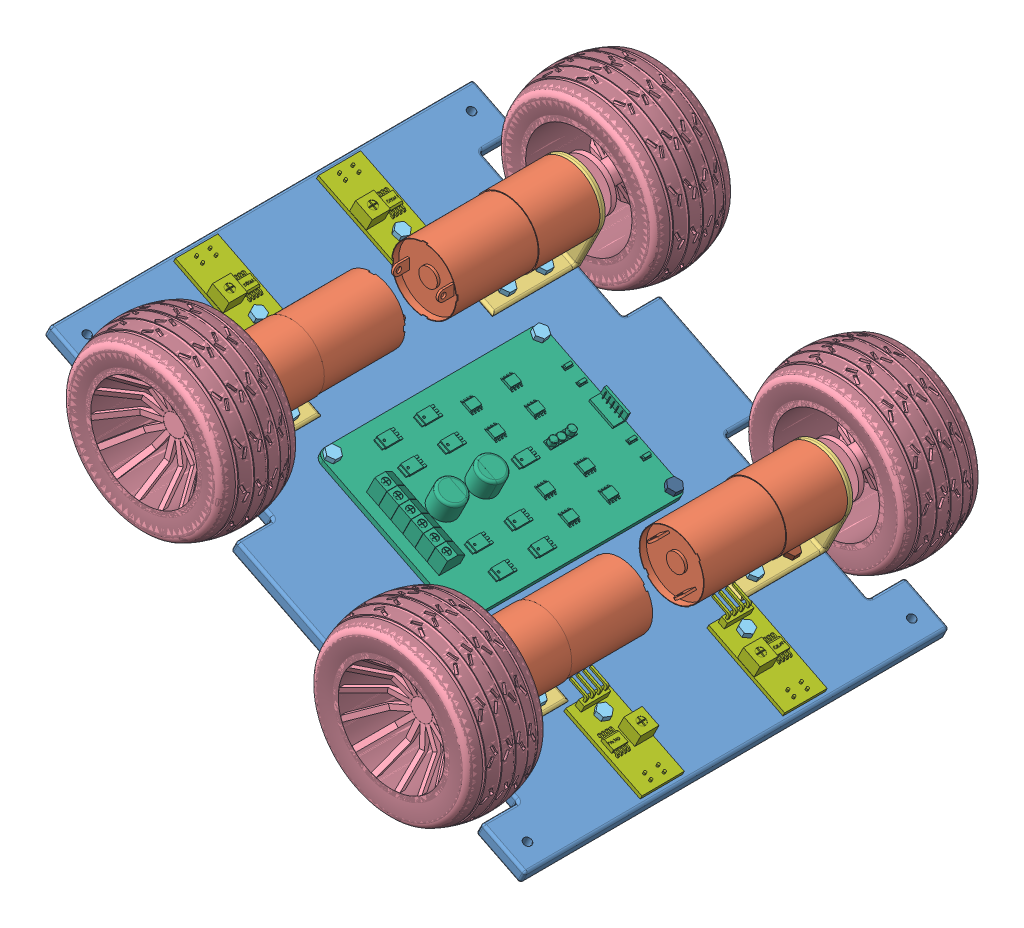
SolidWorks assembly chasse 1 assembly, configuration Default. Lengths in mm.
Overall size (204.59 144.82 194.38).
79 component instances, 12 part files, 19 mates.
Components (placement in the parent):
- down chasse-1: down chasse [Default] at (-215.8058 163.912 27.6173) x (-0.893788 0.448484 0.002276) z (-0.002035 0.001021 -0.999997) size (200 5 160)
- Motor assembly-9: Motor assembly [Default] at (-169.303 117.4456 37.7845) x (-0.59772 0.801702 0.002172) z (-0.002172 0.00109 -0.999997) size (81.67 81.67 90.74)
  - dc motor-1: dc motor [Default] at (29.3048 35.2797 20.0121) size (25 25 72.3)
  - new motor holder-1: new motor holder [Default] at (32.8529 14.4792 73.8121) x (-0.89379 0.448485 0) z (0 0 -1) size (25 31.5 33)
  - tire-2: tire [Défaut] at (29.3048 35.2797 92.3578) x (0 0 -1) z (-0.952681 -0.303972 0) size (29.78 64.99 64.99)
  - bolt-1: bolt [Default] at (36.902 31.4676 76.4477) x (-0.31031 -0.950635 0) z (0 0 -1) size (5.19 4.62 12)
  - bolt-2: bolt [Default] at (21.7075 39.0918 76.1821) x (0.923728 0.383049 0) z (0 0 -1) size (5.19 4.62 12)
- Motor assembly-14: Motor assembly [MirrorDefault] at (-169.345 117.4667 17.166) x (-0.59772 0.801703 0.001897) z (-0.001897 0.000952 -0.999998) size (81.67 81.67 90.74)
  - dc motor-1: dc motor [MirrorDefault] at (29.3048 35.2797 -20.0121) size (25 25 72.3)
  - new motor holder-1: new motor holder [MirrorDefault] at (32.8529 14.4792 -73.8121) x (-0.89379 0.448485 0) z (0 0 -1) size (25 31.5 33)
  - tire-2: tire [MirrorDéfaut] at (29.3048 35.2797 -92.3578) x (0 0 1) z (0.952681 0.303972 0) size (29.78 64.99 64.99)
  - bolt-1: bolt [MirrorDefault] at (36.902 31.4676 -76.4477) x (-0.31031 -0.950635 0) z (0 0 -1) size (5.19 4.62 12)
  - bolt-2: bolt [MirrorDefault] at (21.7075 39.0918 -76.1821) x (0.923728 0.383049 0) z (0 0 -1) size (5.19 4.62 12)
- Motor assembly-15: Motor assembly [MirrorDefault] at (-280.8119 173.3985 38.0686) x (0.999998 0.000001 -0.001897) z (0.001897 -0.000952 0.999998) size (81.67 81.67 90.74)
  - dc motor-1: dc motor [MirrorDefault] at (29.3048 35.2797 -20.0121) size (25 25 72.3)
  - new motor holder-1: new motor holder [MirrorDefault] at (32.8529 14.4792 -73.8121) x (-0.89379 0.448485 0) z (0 0 -1) size (25 31.5 33)
  - tire-2: tire [MirrorDéfaut] at (29.3048 35.2797 -92.3578) x (0 0 1) z (0.952681 0.303972 0) size (29.78 64.99 64.99)
  - bolt-1: bolt [MirrorDefault] at (36.902 31.4676 -76.4477) x (-0.31031 -0.950635 0) z (0 0 -1) size (5.19 4.62 12)
  - bolt-2: bolt [MirrorDefault] at (21.7075 39.0918 -76.1821) x (0.923728 0.383049 0) z (0 0 -1) size (5.19 4.62 12)
- Motor assembly-16: Motor assembly [MirrorMirrorDefault] at (-280.8538 173.4195 17.45) x (0.999998 0.000001 -0.002172) z (0.002172 -0.00109 0.999997) size (81.67 81.67 90.74)
  - dc motor-1: dc motor [MirrorMirrorDefault] at (29.3048 35.2797 20.0121) size (25 25 72.3)
  - new motor holder-1: new motor holder [MirrorMirrorDefault] at (32.8529 14.4792 73.8121) x (-0.89379 0.448485 0) z (0 0 -1) size (25 31.5 33)
  - tire-2: tire [MirrorMirrorDéfaut] at (29.3048 35.2797 92.3578) x (0 0 -1) z (-0.952681 -0.303972 0) size (29.78 64.99 64.99)
  - bolt-1: bolt [MirrorMirrorDefault] at (36.902 31.4676 76.4477) x (-0.31031 -0.950635 0) z (0 0 -1) size (5.19 4.62 12)
  - bolt-2: bolt [MirrorMirrorDefault] at (21.7075 39.0918 76.1821) x (0.923728 0.383049 0) z (0 0 -1) size (5.19 4.62 12)
- Motor Driver-1: Motor Driver [Default] at (-213.5634 168.381 27.6173) x (-0.002035 0.001021 -0.999997) z (0.893788 -0.448484 -0.002276) size (84.5 10.09 62)
- Arduino_HM_proximity_sensor-1: Arduino_HM_proximity_sensor [По умолчанию] at (-153.9567 140.1498 8.4513) x (0.89379 -0.448485 0.000154) z (-0.448485 -0.89379 0) size (37.02 16 16.8)
- Arduino_HM_proximity_sensor-2: Arduino_HM_proximity_sensor [MirrorПо умолчанию] at (-153.8794 140.111 46.4828) x (0.89378 -0.44848 -0.004707) z (0.448485 0.89379 0) size (37.02 16 16.8)
- Arduino_HM_proximity_sensor-3: Arduino_HM_proximity_sensor [MirrorПо умолчанию] at (-271.902 199.3323 8.7517) x (-0.89378 0.44848 0.004707) z (0.448485 0.89379 0) size (37.02 16 16.8)
- Arduino_HM_proximity_sensor-4: Arduino_HM_proximity_sensor [MirrorПо умолчанию] at (-271.8268 199.2946 62.7833) x (-0.89379 0.448485 -0.000154) z (0.448485 0.89379 0) size (37.02 16 16.8)
- Part1^chasse 1 assembly-1: Part1^chasse 1 assembly [Default] at origin (virtual)
- bolt-1: bolt [Default] at (-147.6975 138.1279 0.4523) x (-0.34547 0.17335 -0.92228) z (-0.448485 -0.89379 0) size (5.19 4.62 12)
- nut (1)-1: nut (1) [Default] at (-151.7339 130.0838 0.4523) x (0.798861 -0.400852 -0.448485) z (0.448485 0.89379 0) size (5.28 5.69 3.19)
- Mirrornut (1)-2: Mirrornut (1) [Default] at (-151.624 130.0287 54.4522) x (0.800678 -0.401763 0.444411) z (-0.448485 -0.89379 0) size (5.28 5.69 3.19)
- bolt-2: bolt [Default] at (-147.5876 138.0728 54.4522) x (-0.341714 0.171465 0.92403) z (-0.448485 -0.89379 0) size (5.19 4.62 12)
- Mirrornut (1)-3: Mirrornut (1) [Default] at (-281.3331 195.114 0.7824) x (-0.800678 0.401763 -0.444411) z (-0.448485 -0.89379 0) size (5.28 5.69 3.19)
- bolt-3: bolt [Default] at (-277.2968 203.1581 0.7824) x (0.341714 -0.171465 -0.92403) z (-0.448485 -0.89379 0) size (5.19 4.62 12)
- Mirrornut (1)-4: Mirrornut (1) [Default] at (-281.2235 195.0583 54.7823) x (-0.798861 0.400852 0.448485) z (0.448485 0.89379 0) size (5.28 5.69 3.19)
- bolt-4: bolt [Default] at (-277.1869 203.103 54.7823) x (0.34547 -0.17335 0.92228) z (-0.448485 -0.89379 0) size (5.19 4.62 12)
- bolt-5: bolt [Default] at (-237.279 183.7494 -11.5689) x (0.798861 -0.400852 0.448485) z (-0.448485 -0.89379 0) size (5.19 4.62 12)
- nut (1)-2: nut (1) [Default] at (-241.5918 175.1726 -11.4981) x (0.887126 -0.445142 0.121884) z (-0.448485 -0.89379 0) size (5.28 5.69 3.19)
- Mirrorbolt-6: Mirrorbolt [Default] at (-187.2269 158.6343 -11.6964) x (-0.797028 0.399932 0.45255) z (0.448485 0.89379 0) size (5.19 4.62 12)
- nut (1)-3: nut (1) [Default] at (-191.5245 150.0506 -11.6256) x (-0.886621 0.444888 0.126402) z (0.448485 0.89379 0) size (5.28 5.69 3.19)
- bolt-6: bolt [Default] at (-237.1193 183.6692 66.9309) x (0.797028 -0.399932 -0.45255) z (-0.448485 -0.89379 0) size (5.19 4.62 12)
- nut (1)-4: nut (1) [Default] at (-241.4321 175.0932 66.8601) x (0.886621 -0.444888 -0.126402) z (0.448485 0.89379 0) size (5.28 5.69 3.19)
- Mirrorbolt-7: Mirrorbolt [Default] at (-187.0672 158.5541 66.8034) x (-0.798861 0.400852 -0.448485) z (0.448485 0.89379 0) size (5.19 4.62 12)
- nut (1)-5: nut (1) [Default] at (-191.3654 149.9701 66.7326) x (-0.887126 0.445142 -0.121884) z (-0.448485 -0.89379 0) size (5.28 5.69 3.19)
- bolt-7: bolt [Default] at (-251.4631 190.7548 68.7173) x (0.798861 -0.400852 0.448485) z (-0.448485 -0.89379 0) size (5.19 4.62 12)
- nut (1)-6: nut (1) [Default] at (-255.7218 182.2628 68.7173) x (0.798861 -0.400852 -0.448485) z (0.448485 0.89379 0) size (5.28 5.69 3.19)
- nut (1)-7: nut (1) [Default] at (-255.6933 182.2485 82.7173) x (0.798861 -0.400852 0.448485) z (-0.448485 -0.89379 0) size (5.28 5.69 3.19)
- bolt-8: bolt [Default] at (-251.4327 190.7395 82.7173) x (0.798861 -0.400852 0.448485) z (-0.448485 -0.89379 0) size (5.19 4.62 12)
- nut (1)-8: nut (1) [Default] at (-270.0224 189.4385 68.7538) x (-0.867359 0.435223 -0.24139) z (0.448485 0.89379 0) size (5.28 5.69 3.19)
- bolt-9: bolt [Default] at (-265.7637 197.9305 68.7538) x (0.798861 -0.400852 0.448485) z (-0.448485 -0.89379 0) size (5.19 4.62 12)
- bolt-10: bolt [Default] at (-265.7333 197.9152 82.7537) x (0.798861 -0.400852 0.448485) z (-0.448485 -0.89379 0) size (5.19 4.62 12)
- nut (1)-10: nut (1) [Default] at (-269.9939 189.4242 82.7537) x (0.798861 -0.400852 -0.448485) z (0.448485 0.89379 0) size (5.28 5.69 3.19)
- Mirrorbolt1-12: Mirrorbolt1 [Default] at (-265.9571 198.0276 -27.246) x (0.797028 -0.399932 -0.45255) z (0.448485 0.89379 0) size (5.19 4.62 12)
- bolt-12: bolt [Default] at (-265.9306 198.0142 -13.246) x (0.797028 -0.399932 -0.45255) z (-0.448485 -0.89379 0) size (5.19 4.62 12)
- bolt-13: bolt [Default] at (-251.63 190.8385 -13.2824) x (0.797028 -0.399932 -0.45255) z (-0.448485 -0.89379 0) size (5.19 4.62 12)
- bolt-14: bolt [Default] at (-251.6565 190.8518 -27.2824) x (0.797028 -0.399932 -0.45255) z (-0.448485 -0.89379 0) size (5.19 4.62 12)
- nut (1)-11: nut (1) [Default] at (-255.9169 182.3613 -27.2824) x (0.797028 -0.399932 -0.45255) z (0.448485 0.89379 0) size (5.28 5.69 3.19)
- nut (1)-12: nut (1) [Default] at (-270.218 189.536 -27.246) x (0.800678 -0.401763 0.444411) z (-0.448485 -0.89379 0) size (5.28 5.69 3.19)
- nut (1)-13: nut (1) [Default] at (-270.1895 189.5217 -13.246) x (-0.866368 0.434725 0.245806) z (-0.448485 -0.89379 0) size (5.28 5.69 3.19)
- nut (1)-14: nut (1) [Default] at (-255.8889 182.346 -13.2824) x (0.800678 -0.401763 0.444411) z (-0.448485 -0.89379 0) size (5.28 5.69 3.19)
- Mirrorbolt-15: Mirrorbolt [Default] at (-158.4788 144.0972 82.4805) x (-0.797028 0.399932 0.45255) z (0.448485 0.89379 0) size (5.19 4.62 12)
- bolt-15: bolt [Default] at (-158.5053 144.1105 68.4806) x (-0.797028 0.399932 0.45255) z (-0.448485 -0.89379 0) size (5.19 4.62 12)
- bolt-16: bolt [Default] at (-172.8059 151.2862 68.517) x (-0.797028 0.399932 0.45255) z (-0.448485 -0.89379 0) size (5.19 4.62 12)
- bolt-17: bolt [Default] at (-172.7794 151.2729 82.517) x (-0.797028 0.399932 0.45255) z (-0.448485 -0.89379 0) size (5.19 4.62 12)
- nut (1)-15: nut (1) [Default] at (-177.0397 142.7824 82.517) x (-0.797028 0.399932 0.45255) z (0.448485 0.89379 0) size (5.28 5.69 3.19)
- nut (1)-16: nut (1) [Default] at (-162.7397 135.6056 82.4805) x (-0.800678 0.401763 -0.444411) z (-0.448485 -0.89379 0) size (5.28 5.69 3.19)
- nut (1)-17: nut (1) [Default] at (-162.7681 135.6199 68.4806) x (0.866368 -0.434725 -0.245806) z (-0.448485 -0.89379 0) size (5.28 5.69 3.19)
- nut (1)-18: nut (1) [Default] at (-177.0687 142.7956 68.517) x (-0.800678 0.401763 -0.444411) z (-0.448485 -0.89379 0) size (5.28 5.69 3.19)
- Mirrorbolt1-13: Mirrorbolt1 [Default] at (-158.7026 144.2095 -27.5192) x (-0.798861 0.400852 -0.448485) z (0.448485 0.89379 0) size (5.19 4.62 12)
- bolt-18: bolt [Default] at (-158.6722 144.1942 -13.5192) x (-0.798861 0.400852 -0.448485) z (-0.448485 -0.89379 0) size (5.19 4.62 12)
- bolt-19: bolt [Default] at (-172.9728 151.3699 -13.4828) x (-0.798861 0.400852 -0.448485) z (-0.448485 -0.89379 0) size (5.19 4.62 12)
- bolt-20: bolt [Default] at (-173.0032 151.3852 -27.4827) x (-0.798861 0.400852 -0.448485) z (-0.448485 -0.89379 0) size (5.19 4.62 12)
- nut (1)-19: nut (1) [Default] at (-177.2638 142.8942 -27.4827) x (-0.798861 0.400852 -0.448485) z (-0.448485 -0.89379 0) size (5.28 5.69 3.19)
- nut (1)-20: nut (1) [Default] at (-162.9632 135.7185 -27.5192) x (-0.798861 0.400852 0.448485) z (0.448485 0.89379 0) size (5.28 5.69 3.19)
- nut (1)-21: nut (1) [Default] at (-162.9347 135.7042 -13.5192) x (0.867359 -0.435223 0.24139) z (0.448485 0.89379 0) size (5.28 5.69 3.19)
- nut (1)-22: nut (1) [Default] at (-177.2353 142.8799 -13.4828) x (-0.798861 0.400852 0.448485) z (0.448485 0.89379 0) size (5.28 5.69 3.19)
Mates (geometry in assembly coordinates):
- Coincident18: coincident aligned: circle of down chasse-1; circle of Motor assembly-9/new motor holder-1
- Coincident19: coincident aligned: circle of down chasse-1; circle of Motor assembly-9/new motor holder-1
- Concentric3: concentric aligned: circle of down chasse-1; circle of Motor assembly-9/new motor holder-1
- Coincident23: coincident aligned: circle of down chasse-1; circle of Motor Driver-1
- Coincident24: coincident aligned: circle of down chasse-1; circle of Motor Driver-1
- Coincident47: coincident anti-aligned: circle of down chasse-1; circle of Arduino_HM_proximity_sensor-1
- Coincident48: coincident aligned: circle of Arduino_HM_proximity_sensor-1; circle of bolt-1
- Coincident49: coincident anti-aligned: line of bolt-1 through (-152.4066 128.7431 0.4523) axis (0.448485 0.89379 0); line of nut (1)-1 through (-151.0612 131.4245 0.4523) axis (-0.448485 -0.89379 0)
- Coincident50: coincident aligned: circle of down chasse-1; circle of nut (1)-1
- Coincident51: coincident anti-aligned: circle of Motor Driver-1; circle of bolt-5
- Tangent2: tangent: curve of down chasse-1; curve of nut (1)-2
- Coincident53: coincident anti-aligned: circle of Motor assembly-16/new motor holder-1; circle of bolt-7
- Coincident56: coincident anti-aligned: circle of Motor assembly-16/new motor holder-1; circle of bolt-8
- Coincident57: coincident anti-aligned: circle of Motor assembly-16/new motor holder-1; circle of bolt-9
- Coincident58: coincident anti-aligned: circle of Motor assembly-16/new motor holder-1; circle of bolt-10
- Coincident59: coincident anti-aligned: circle of down chasse-1; circle of nut (1)-7
- Coincident60: coincident aligned: circle of down chasse-1; circle of nut (1)-8
- Coincident61: coincident anti-aligned: line of down chasse-1 through (-269.3212 190.7649 82.7537) axis (0.448485 0.89379 0); line of nut (1)-10 through (-269.3212 190.7649 82.7537) axis (-0.448485 -0.89379 0)
- Coincident62: coincident anti-aligned: line of down chasse-1 through (-255.0491 183.6035 68.7173) axis (0.448485 0.89379 0); line of nut (1)-6 through (-255.0491 183.6035 68.7173) axis (-0.448485 -0.89379 0)
